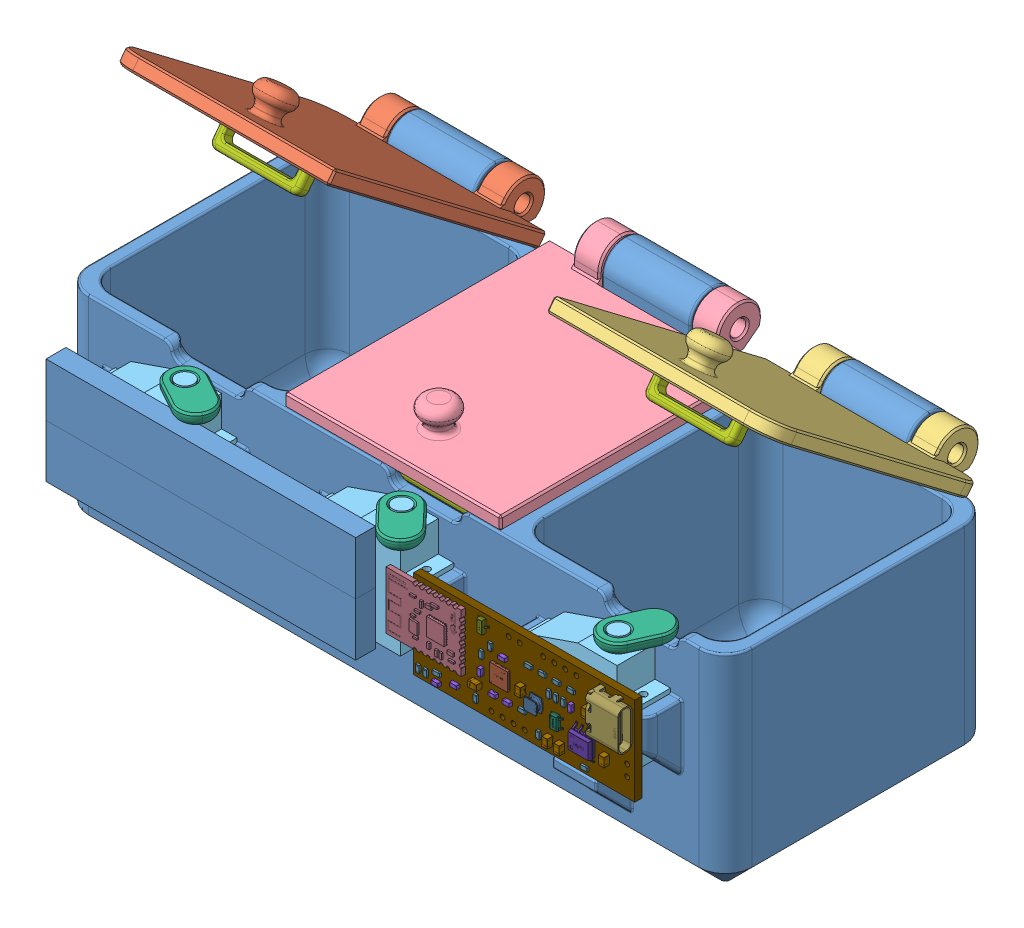
SolidWorks assembly 装配, configuration 默认. Lengths in mm.
Overall size (150 94.48 83.55).
139 component instances, 22 part files, 42 mates.
Components (placement in the parent):
- 盒子-1: 盒子 [默认] at (-79.9939 -35.3926 182.681) size (150 58 75.91)
- 边盖-1: 边盖 [默认] at (-29.4939 51.285 172.8919) x (0 -0.604443 -0.796648) z (1 0 0) size (67.2 9.8 50.35)
- 镜向边盖-2: 镜向边盖 [默认] at (19.5061 51.285 172.8919) x (0 -0.604443 -0.796648) z (1 0 0) size (67.2 9.8 50.35)
- 中盖-1: 中盖 [默认] at (19.3061 12.7974 182.671) x (0 0 -1) z (1 0 0) size (67.2 9.8 48.9)
- 小舵机-1: 小舵机 [默认] at (-64.3939 -14.1926 191.281) size (27.5 25.65 8.6)
- 小舵机-2: 小舵机 [默认] at (33.6061 -14.1926 191.281) size (27.5 25.65 8.6)
- 小舵机-3: 小舵机 [默认] at (-15.3939 -14.1926 191.281) size (27.5 25.65 8.6)
- 锁-1: 锁 [默认] at (-47.8939 8.4574 186.981) x (0 1 0) z (0.479802 0 -0.877377) size (3 14 8)
- 锁-2: 锁 [默认] at (50.1061 8.4574 186.981) x (0 1 0) z (-0.912479 0 -0.409122) size (3 14 8)
- 锁-3: 锁 [默认] at (1.1061 8.4574 186.981) x (0 1 0) z (0.725826 0 -0.687879) size (3 14 8)
- 电路盒-1: 电路盒 [默认] at (64.0061 -30.3926 200.181) x (-1 0 0) z (0 0 -1) size (138 47.35 22.96) (hidden)
- 盖子锁口-1: 盖子锁口 [默认] at (-56.9939 43.6916 170.4941) x (1 0 0) z (0 -0.796648 0.604443) size (20 3 6.1)
- 盖子锁口-2: 盖子锁口 [默认] at (41.0061 43.6916 170.4941) x (1 0 0) z (0 -0.796648 0.604443) size (20 3 6.1)
- 盖子锁口-3: 盖子锁口 [默认] at (-7.9939 8.1974 176.171) x (1 0 0) z (0 -1 0) size (20 3 6.1)
- 3D_BOX_2024-11-24-1: 3D_BOX_2024-11-24 [默认] at (10.7267 5.7947 191.781) size (55.21 19.97 4.86)
  - 3D_BOX_2024-11-24.step-1: 3D_BOX_2024-11-24.step [默认] at origin size (56.98 23.31 10.6)
    - 3yDE-C2.step-1: 3yDE-C2.step [默认] at (21.082 -14.478 1.6001) x (-1 0 0) z (0 0 1) size (1.6 0.8 0.8)
      - C0603.step-1: C0603.step [默认] at origin size (1.6 0.8 0.8)
        - SOLID.step-1: SOLID.step [默认] at origin size (1.6 0.8 0.8)
    - 3yDE-C3.step-1: 3yDE-C3.step [默认] at (14.986 -11.43 1.6001) x (0 -1 0) z (0 0 1) size (1.6 0.8 0.8)
      - C0603.step-1: C0603.step [默认] at origin size (1.6 0.8 0.8)
        - SOLID.step-1: SOLID.step [默认] at origin size (1.6 0.8 0.8)
    - 3yDE-C4.step-1: 3yDE-C4.step [默认] at (20.066 -6.223 1.6001) x (-1 0 0) z (0 0 1) size (1.6 0.8 0.8)
      - C0603.step-1: C0603.step [默认] at origin size (1.6 0.8 0.8)
        - SOLID.step-1: SOLID.step [默认] at origin size (1.6 0.8 0.8)
    - 3yDE-C5.step-1: 3yDE-C5.step [默认] at (9.144 -17.018 1.6001) x (-1 0 0) z (0 0 1) size (1.6 0.8 0.8)
      - C0603.step-1: C0603.step [默认] at origin size (1.6 0.8 0.8)
        - SOLID.step-1: SOLID.step [默认] at origin size (1.6 0.8 0.8)
    - 3yDE-C6.step-1: 3yDE-C6.step [默认] at (4.953 -18.669 1.6001) x (-1 0 0) z (0 0 1) size (1.6 0.8 0.8)
      - C0603.step-1: C0603.step [默认] at origin size (1.6 0.8 0.8)
        - SOLID.step-1: SOLID.step [默认] at origin size (1.6 0.8 0.8)
    - 3yDE-C11.step-1: 3yDE-C11.step [默认] at (35.4331 -8.255 1.6001) x (0 -1 0) z (0 0 1) size (1.6 0.8 0.8)
      - C0603.step-1: C0603.step [默认] at origin size (1.6 0.8 0.8)
        - SOLID.step-1: SOLID.step [默认] at origin size (1.6 0.8 0.8)
    - 3yDE-C1.step-1: 3yDE-C1.step [默认] at (17.907 -14.478 1.6001) size (1.6 0.8 0.8)
      - C0603.step-1: C0603.step [默认] at origin size (1.6 0.8 0.8)
        - SOLID.step-1: SOLID.step [默认] at origin size (1.6 0.8 0.8)
    - 3yDE-C8.step-1: 3yDE-C8.step [默认] at (24.257 -10.287 1.6001) x (0 -1 0) z (0 0 1) size (2 1.3 1.3)
      - C0805.step-1: C0805.step [默认] at origin size (2 1.3 1.3)
        - SOLID-0.step-1: SOLID-0.step [默认] at origin size (2 1.3 1.3)
    - 3yDE-C9.step-1: 3yDE-C9.step [默认] at (33.0201 -17.272 1.6001) x (0 1 0) z (0 0 1) size (2 1.3 1.3)
      - C0805.step-1: C0805.step [默认] at origin size (2 1.3 1.3)
        - SOLID-0.step-1: SOLID-0.step [默认] at origin size (2 1.3 1.3)
    - 3yDE-C10.step-1: 3yDE-C10.step [默认] at (30.3531 -17.272 1.6001) x (0 1 0) z (0 0 1) size (2 1.3 1.3)
      - C0805.step-1: C0805.step [默认] at origin size (2 1.3 1.3)
        - SOLID-0.step-1: SOLID-0.step [默认] at origin size (2 1.3 1.3)
    - 3yDE-C12.step-1: 3yDE-C12.step [默认] at (39.2431 -7.112 1.6001) x (0 -1 0) z (0 0 1) size (2 1.3 1.3)
      - C0805.step-1: C0805.step [默认] at origin size (2 1.3 1.3)
        - SOLID-0.step-1: SOLID-0.step [默认] at origin size (2 1.3 1.3)
    - 3yDE-C13.step-1: 3yDE-C13.step [默认] at (43.1801 -14.478 1.6001) x (0 1 0) z (0 0 1) size (2 1.3 1.3)
      - C0805.step-1: C0805.step [默认] at origin size (2 1.3 1.3)
        - SOLID-0.step-1: SOLID-0.step [默认] at origin size (2 1.3 1.3)
    - 3yDE-C7.step-1: 3yDE-C7.step [默认] at (13.97 -14.351 1.6001) x (-1 0 0) z (0 0 1) size (2 1.3 1.3)
      - C0805.step-1: C0805.step [默认] at origin size (2 1.3 1.3)
        - SOLID-0.step-1: SOLID-0.step [默认] at origin size (2 1.3 1.3)
    - 3yDE-S1.step-1: 3yDE-S1.step [默认] at (32.5121 -1.778 1.6001) size (12.5 5.7 10)
      - CONN-TH_4P-P2.50_4PIN.step-1: CONN-TH_4P-P2.50_4PIN.step [默认] at origin size (12.5 5.7 10)
        - COMPOUND.step-1: COMPOUND.step [默认] at origin size (12.5 5.7 10) (hidden)
    - 3yDE-DOWNLOAD1.step-1: 3yDE-DOWNLOAD1.step [默认] at (20.828 -18.288 1.6001) x (-1 0 0) z (0 0 1) size (12.5 5.7 10)
      - CONN-TH_4P-P2.50_4PIN.step-1: CONN-TH_4P-P2.50_4PIN.step [默认] at origin size (12.5 5.7 10)
        - COMPOUND.step-1: COMPOUND.step [默认] at origin size (12.5 5.7 10) (hidden)
    - 3yDE-L1.step-1: 3yDE-L1.step [默认] at (27.3051 -11.557 1.6001) x (0 -1 0) z (0 0 1) size (3 3 1.52)
      - IND-SMD_L3.0-W3.0_FNR30XXS.step-1: IND-SMD_L3.0-W3.0_FNR30XXS.step [默认] at origin size (3 3 1.52)
        - SOLID-1.step-1: SOLID-1.step [默认] at origin size (3 3 1.52)
    - 3yDE-U2.step-1: 3yDE-U2.step [默认] at (19.304 -10.287 1.6001) size (4.03 4.03 0.61)
      - UFQFPN-28_L4.0-W4.0-P0.50-BL.step-1: UFQFPN-28_L4.0-W4.0-P0.50-BL.step [默认] at origin size (4.03 4.03 0.61)
        - SOLID-2.step-1: SOLID-2.step [默认] at origin size (4.03 4.03 0.61)
    - 3yDE-BAT1.step-1: 3yDE-BAT1.step [默认] at (47.7521 -14.605 1.6001) x (0 1 0) z (0 0 1) size (7.5 5.9 10.6)
      - CONN-TH_2P-P2.50_HX25003-2A.step-1: CONN-TH_2P-P2.50_HX25003-2A.step [默认] at origin size (7.5 5.9 10.6)
        - COMPOUND-3.step-1: COMPOUND-3.step [默认] at origin size (7.5 5.9 10.6) (hidden)
    - 3yDE-SPOWER1.step-1: 3yDE-SPOWER1.step [默认] at (22.225 -1.778 1.6001) x (-1 0 0) z (0 0 1) size (7.5 5.9 10.6)
      - CONN-TH_2P-P2.50_HX25003-2A.step-1: CONN-TH_2P-P2.50_HX25003-2A.step [默认] at origin size (7.5 5.9 10.6)
        - COMPOUND-3.step-1: COMPOUND-3.step [默认] at origin size (7.5 5.9 10.6) (hidden)
    - 3yDE-USB1.step-1: 3yDE-USB1.step [默认] at (43.9421 -5.334 1.6001) x (0 1 0) z (0 0 1) size (8.95 7.58 4.16)
      - USB-C-SMD_TYPE-C-6PIN-2MD-073.step-1: USB-C-SMD_TYPE-C-6PIN-2MD-073.step [默认] at origin size (8.95 7.58 4.16)
        - COMPOUND-4.step-1: COMPOUND-4.step [默认] at origin size (8.95 7.58 4.16)
    - 3yDE-U1.step-1: 3yDE-U1.step [默认] at (5.969 -7.493 1.6001) x (0 1 0) z (0 0 1) size (13 17 1.62)
      - BULETM-SMD_ZX-D30.step-1: BULETM-SMD_ZX-D30.step [默认] at origin size (13 17 1.62)
        - SOLID-5.step-1: SOLID-5.step [默认] at origin size (13 17 1.62)
    - 3yDE-R2.step-1: 3yDE-R2.step [默认] at (24.2672 -14.4989 1.6001) x (-1 0 0) z (0 0 1) size (1.62 0.81 0.45)
      - R0603.step-1: R0603.step [默认] at origin size (1.62 0.81 0.45)
        - COMPOUND-6.step-1: COMPOUND-6.step [默认] at origin size (1.62 0.81 0.45)
    - 3yDE-R3.step-1: 3yDE-R3.step [默认] at (4.953 -16.891 1.6001) x (-1 0 0) z (0 0 1) size (1.62 0.81 0.45)
      - R0603.step-1: R0603.step [默认] at origin size (1.62 0.81 0.45)
        - COMPOUND-6.step-1: COMPOUND-6.step [默认] at origin size (1.62 0.81 0.45)
    - 3yDE-R4.step-1: 3yDE-R4.step [默认] at (0.762 -18.034 1.6001) x (0 1 0) z (0 0 1) size (1.62 0.81 0.45)
      - R0603.step-1: R0603.step [默认] at origin size (1.62 0.81 0.45)
        - COMPOUND-6.step-1: COMPOUND-6.step [默认] at origin size (1.62 0.81 0.45)
    - 3yDE-R5.step-1: 3yDE-R5.step [默认] at (2.413 -18.034 1.6001) x (0 1 0) z (0 0 1) size (1.62 0.81 0.45)
      - R0603.step-1: R0603.step [默认] at origin size (1.62 0.81 0.45)
        - COMPOUND-6.step-1: COMPOUND-6.step [默认] at origin size (1.62 0.81 0.45)
    - 3yDE-R6.step-1: 3yDE-R6.step [默认] at (13.716 -17.399 1.6001) x (0 1 0) z (0 0 1) size (1.62 0.81 0.45)
      - R0603.step-1: R0603.step [默认] at origin size (1.62 0.81 0.45)
        - COMPOUND-6.step-1: COMPOUND-6.step [默认] at origin size (1.62 0.81 0.45)
    - 3yDE-R7.step-1: 3yDE-R7.step [默认] at (27.9401 -17.399 1.6001) x (0 1 0) z (0 0 1) size (1.62 0.81 0.45)
      - R0603.step-1: R0603.step [默认] at origin size (1.62 0.81 0.45)
        - COMPOUND-6.step-1: COMPOUND-6.step [默认] at origin size (1.62 0.81 0.45)
    - 3yDE-R8.step-1: 3yDE-R8.step [默认] at (35.3061 -5.08 1.6001) x (-1 0 0) z (0 0 1) size (1.62 0.81 0.45)
      - R0603.step-1: R0603.step [默认] at origin size (1.62 0.81 0.45)
        - COMPOUND-6.step-1: COMPOUND-6.step [默认] at origin size (1.62 0.81 0.45)
    - 3yDE-R9.step-1: 3yDE-R9.step [默认] at (32.0041 -5.08 1.6001) x (-1 0 0) z (0 0 1) size (1.62 0.81 0.45)
      - R0603.step-1: R0603.step [默认] at origin size (1.62 0.81 0.45)
        - COMPOUND-6.step-1: COMPOUND-6.step [默认] at origin size (1.62 0.81 0.45)
    - 3yDE-R10.step-1: 3yDE-R10.step [默认] at (28.8291 -5.08 1.6001) x (-1 0 0) z (0 0 1) size (1.62 0.81 0.45)
      - R0603.step-1: R0603.step [默认] at origin size (1.62 0.81 0.45)
        - COMPOUND-6.step-1: COMPOUND-6.step [默认] at origin size (1.62 0.81 0.45)
    - 3yDE-R11.step-1: 3yDE-R11.step [默认] at (25.6541 -5.08 1.6001) x (-1 0 0) z (0 0 1) size (1.62 0.81 0.45)
      - R0603.step-1: R0603.step [默认] at origin size (1.62 0.81 0.45)
        - COMPOUND-6.step-1: COMPOUND-6.step [默认] at origin size (1.62 0.81 0.45)
    - 3yDE-R12.step-1: 3yDE-R12.step [默认] at (30.2261 -8.255 1.6001) x (0 -1 0) z (0 0 1) size (1.62 0.81 0.45)
      - R0603.step-1: R0603.step [默认] at origin size (1.62 0.81 0.45)
        - COMPOUND-6.step-1: COMPOUND-6.step [默认] at origin size (1.62 0.81 0.45)
    - 3yDE-R13.step-1: 3yDE-R13.step [默认] at (31.8771 -8.255 1.6001) x (0 1 0) z (0 0 1) size (1.62 0.81 0.45)
      - R0603.step-1: R0603.step [默认] at origin size (1.62 0.81 0.45)
        - COMPOUND-6.step-1: COMPOUND-6.step [默认] at origin size (1.62 0.81 0.45)
    - 3yDE-R16.step-1: 3yDE-R16.step [默认] at (38.3541 -18.669 1.6001) x (-1 0 0) z (0 0 1) size (1.62 0.81 0.45)
      - R0603.step-1: R0603.step [默认] at origin size (1.62 0.81 0.45)
        - COMPOUND-6.step-1: COMPOUND-6.step [默认] at origin size (1.62 0.81 0.45)
    - 3yDE-R17.step-1: 3yDE-R17.step [默认] at (17.018 -5.588 1.6001) x (0 1 0) z (0 0 1) size (1.62 0.81 0.45)
      - R0603.step-1: R0603.step [默认] at origin size (1.62 0.81 0.45)
        - COMPOUND-6.step-1: COMPOUND-6.step [默认] at origin size (1.62 0.81 0.45)
    - 3yDE-R14.step-1: 3yDE-R14.step [默认] at (33.5281 -8.255 1.6001) x (0 -1 0) z (0 0 1) size (1.62 0.81 0.45)
      - R0603.step-1: R0603.step [默认] at origin size (1.62 0.81 0.45)
        - COMPOUND-6.step-1: COMPOUND-6.step [默认] at origin size (1.62 0.81 0.45)
    - 3yDE-R1.step-1: 3yDE-R1.step [默认] at (14.986 -8.128 1.6001) x (0 -1 0) z (0 0 1) size (1.62 0.81 0.45)
      - R0603.step-1: R0603.step [默认] at origin size (1.62 0.81 0.45)
        - COMPOUND-6.step-1: COMPOUND-6.step [默认] at origin size (1.62 0.81 0.45)
    - 3yDE-U3.step-1: 3yDE-U3.step [默认] at (32.0041 -12.7 1.6001) x (0 -1 0) z (0 0 1) size (2.9 2.81 1.05)
      - TSOT-25_L2.9-W1.6-P0.95-BL.step-1: TSOT-25_L2.9-W1.6-P0.95-BL.step [默认] at origin size (2.9 2.81 1.05)
        - COMPOUND-7.step-1: COMPOUND-7.step [默认] at origin size (2.9 2.81 1.05)
    - 3yDE-Q1.step-1: 3yDE-Q1.step [默认] at (15.367 -2.159 1.6001) x (-1 0 0) z (0 0 1) size (2.5 2.89 1.05)
      - SOT-23-3_L2.9-W1.3-P1.90-LS2.4-BR.step-1: SOT-23-3_L2.9-W1.3-P1.90-LS2.4-BR.step [默认] at origin size (2.5 2.89 1.05)
        - COMPOUND-8.step-1: COMPOUND-8.step [默认] at origin size (2.5 2.89 1.05)
    - 3yDE-U4.step-1: 3yDE-U4.step [默认] at (38.3541 -13.716 1.6001) size (4.9 6.1 1.7)
      - ESOP-8_L4.9-W3.9-P1.27-LS6.0-BL-EP.step-1: ESOP-8_L4.9-W3.9-P1.27-LS6.0-BL-EP.step [默认] at origin size (4.9 6.1 1.7)
        - COMPOUND-9.step-1: COMPOUND-9.step [默认] at origin size (4.9 6.1 1.7)
    - Board.step-1: Board.step [默认] at origin size (49.97 19.97 1.6)
- 电池-1: 电池 [默认] at (-70.4939 8.4574 195.781) x (1 0 0) z (0 1 0) size (70 4.5 12)
- 电池-2: 电池 [默认] at (-70.4939 -3.5426 195.781) x (1 0 0) z (0 1 0) size (70 4.5 12)
Mates (geometry in assembly coordinates):
- 重合2: coincident aligned: plane of 盒子-1 through (-79.9939 -32.3926 182.681) normal (-1 0 0); plane of 边盖-1 through (-79.9939 53.675 171.0785) normal (-1 0 0)
- 同心1: concentric anti-aligned: cylinder of 盒子-1 through (70.0061 17.5074 120.581) axis (-1 0 0) radius 1.5; cylinder of 边盖-1 through (-79.9939 17.5074 120.581) axis (1 0 0) radius 1.8
- 同心2: concentric anti-aligned: cylinder of 盒子-1 through (70.0061 17.5074 120.581) axis (-1 0 0) radius 1.5; cylinder of 中盖-1 through (-31.1939 17.5074 120.581) axis (1 0 0) radius 1.8
- 距离1: distance = 0.1 mm anti-aligned: plane of 中盖-1 through (5.1061 5.7974 122.671) normal (-1 0 0); plane of 盒子-1 through (5.0061 22.6074 122.681) normal (1 0 0)
- LimitAngle1: limit planar angle = 0.649066 rad anti-aligned: plane of 边盖-1 through (-29.4939 51.285 172.8919) normal (0 -0.796648 0.604443); plane of 盒子-1 through (-79.9939 12.6074 182.681) normal (0 1 0)
- LimitAngle2: limit planar angle = 0 rad anti-aligned: plane of 中盖-1 through (19.3061 12.7974 182.671) normal (0 -1 0); plane of 盒子-1 through (-79.9939 12.6074 182.681) normal (0 1 0)
- 重合6: coincident anti-aligned: plane of 盒子-1 through (-79.9939 -32.3926 182.681) normal (0 0 1); plane of 小舵机-1 through (-64.3939 1.0074 182.681) normal (0 0 -1)
- 重合7: coincident anti-aligned: plane of 盒子-1 through (-64.4939 0.5074 191.281) normal (0 1 0); plane of 小舵机-1 through (-64.3939 0.5074 182.681) normal (0 -1 0)
- 距离2: distance = 0.1 mm anti-aligned: plane of 小舵机-1 through (-43.8939 1.0074 191.281) normal (1 0 0); plane of 盒子-1 through (-43.7939 0.5074 191.281) normal (-1 0 0)
- 重合9: coincident anti-aligned: plane of 盒子-1 through (5.2061 0.5074 191.281) normal (0 1 0); plane of 小舵机-3 through (5.1061 0.5074 182.681) normal (0 -1 0)
- 同心3: concentric aligned: circle of 盒子-1; cylinder of 小舵机-3 through (6.7261 -7.0926 186.981) axis (0 1 0) radius 0.8
- 同心4: concentric aligned: cylinder of 盒子-1 through (-17.0139 -7.4926 186.981) axis (0 1 0) radius 0.7; cylinder of 小舵机-3 through (-17.0139 -7.0926 186.981) axis (0 1 0) radius 0.8
- 重合10: coincident anti-aligned: plane of 盒子-1 through (33.5061 0.5074 191.281) normal (0 1 0); plane of 小舵机-2 through (54.1061 0.5074 182.681) normal (0 -1 0)
- 同心5: concentric aligned: circle of 盒子-1; circle of 小舵机-2
- 同心6: concentric aligned: cylinder of 盒子-1 through (31.9861 -7.4926 186.981) axis (0 1 0) radius 0.7; cylinder of 小舵机-2 through (31.9861 -7.0926 186.981) axis (0 1 0) radius 0.8
- 同心7: concentric aligned: cylinder of 小舵机-1 through (-47.8939 11.4574 186.981) axis (0 -1 0) radius 2; cylinder of 锁-1 through (-47.8939 11.4574 186.981) axis (0 -1 0) radius 2
- 重合12: coincident anti-aligned: plane of 小舵机-3 through (5.1061 8.4574 182.681) normal (0 1 0); plane of 锁-3 through (1.1061 8.4574 186.981) normal (0 -1 0)
- 重合13: coincident anti-aligned: plane of 小舵机-2 through (54.1061 8.4574 182.681) normal (0 1 0); plane of 锁-2 through (50.1061 8.4574 186.981) normal (0 -1 0)
- 同心8: concentric aligned: cylinder of 小舵机-2 through (50.1061 11.4574 186.981) axis (0 -1 0) radius 2; cylinder of 锁-2 through (50.1061 11.4574 186.981) axis (0 -1 0) radius 2
- 同心9: concentric aligned: cylinder of 小舵机-3 through (1.1061 11.4574 186.981) axis (0 -1 0) radius 2; cylinder of 锁-3 through (1.1061 11.4574 186.981) axis (0 -1 0) radius 2
- 重合14: coincident anti-aligned: plane of 盒子-1 through (-79.9939 -32.3926 182.681) normal (0 0 1); plane of 电路盒-1 through (64.0061 -30.3926 182.681) normal (0 0 -1)
- 重合15: coincident: line of 盒子-1 through (-73.9939 -30.3926 182.681) axis (1 0 0); plane of 电路盒-1 through (64.0061 -30.3926 197.181) normal (0 -1 0)
- 重合16: coincident anti-aligned: line of 盒子-1 through (64.0061 -30.3926 182.681) axis (0 1 0); line of 电路盒-1 through (64.0061 9.0174 182.681) axis (0 -1 0)
- 重合17: coincident aligned: plane of 锁-1 through (-47.8939 11.4574 186.981) normal (0 1 0); plane of 锁-3 through (1.1061 11.4574 186.981) normal (0 1 0)
- 重合18: coincident anti-aligned: plane of 边盖-1 through (-29.4939 52.48 171.9852) normal (0 -0.796648 0.604443); plane of 盖子锁口-1 through (-56.9939 50.3645 169.1969) normal (0 0.796648 -0.604443)
- 距离4: distance = 0.1 mm anti-aligned: plane of 盖子锁口-1 through (-36.9939 45.5049 172.884) normal (1 0 0); plane of 边盖-1 through (-36.8939 50.4249 169.2766) normal (-1 0 0)
- 距离5: distance = 0.1 mm anti-aligned: plane of 盖子锁口-1 through (-56.9939 45.5049 172.884) normal (0 0.604443 0.796648); plane of 边盖-1 through (-57.0939 50.4249 169.2766) normal (0 -0.604443 -0.796648)
- 距离6: distance = 0.1 mm anti-aligned: plane of 盖子锁口-2 through (41.0061 45.5049 172.884) normal (0 0.604443 0.796648); plane of 镜向边盖-2 through (61.1061 50.4249 169.2766) normal (0 -0.604443 -0.796648)
- 距离7: distance = 0.1 mm anti-aligned: plane of 盖子锁口-2 through (61.0061 45.5049 172.884) normal (1 0 0); plane of 镜向边盖-2 through (61.1061 50.4249 169.2766) normal (-1 0 0)
- 重合24: coincident anti-aligned: plane of 镜向边盖-2 through (19.5061 52.48 171.9852) normal (0 -0.796648 0.604443); plane of 盖子锁口-2 through (41.0061 50.3645 169.1969) normal (0 0.796648 -0.604443)
- 重合25: coincident anti-aligned: plane of 中盖-1 through (19.3061 14.2974 182.671) normal (0 -1 0); plane of 盖子锁口-3 through (-7.9939 14.2974 179.171) normal (0 1 0)
- 距离8: distance = 0.1 mm anti-aligned: plane of 盖子锁口-3 through (-7.9939 8.1974 179.171) normal (0 0 1); plane of 中盖-1 through (-8.0939 14.2974 179.271) normal (0 0 -1)
- 距离9: distance = 0.1 mm anti-aligned: plane of 盖子锁口-3 through (12.0061 8.1974 179.171) normal (1 0 0); plane of 中盖-1 through (12.1061 14.2974 179.271) normal (-1 0 0)
- 距离10: distance = 0.5 mm anti-aligned: plane of 小舵机-3 through (-15.3939 1.0074 191.281) normal (0 0 1); plane of 3D_BOX_2024-11-24-1/3D_BOX_2024-11-24.step-1/Board.step-1 through (35.2187 -4.2053 191.781) normal (0 0 -1)
- 重合27: coincident aligned: plane of 盒子-1 through (60.2061 0.5074 191.281) normal (1 0 0); plane of 3D_BOX_2024-11-24-1/3D_BOX_2024-11-24.step-1/Board.step-1 through (60.2061 5.782 191.781) normal (1 0 0)
- 重合28: coincident aligned: plane of 小舵机-2 through (33.6061 -14.1926 191.281) normal (0 -1 0); plane of 3D_BOX_2024-11-24-1/3D_BOX_2024-11-24.step-1/Board.step-1 through (60.2061 -14.1926 191.781) normal (0 -1 0)
- 重合29: coincident anti-aligned: plane of 小舵机-1 through (-64.3939 1.0074 191.281) normal (0 0 1); plane of 电池-1 through (-70.4939 8.4574 191.281) normal (0 0 -1)
- 重合30: coincident anti-aligned: plane of 小舵机-1 through (-64.3939 1.0074 191.281) normal (0 0 1); plane of 电池-2 through (-70.4939 -3.5426 191.281) normal (0 0 -1)
- 重合32: coincident aligned: plane of 盒子-1 through (-70.4939 0.5074 191.281) normal (-1 0 0); plane of 电池-1 through (-70.4939 8.4574 191.281) normal (-1 0 0)
- 重合33: coincident aligned: plane of 盒子-1 through (-70.4939 0.5074 191.281) normal (-1 0 0); plane of 电池-2 through (-70.4939 -3.5426 191.281) normal (-1 0 0)
- 重合34: coincident aligned: plane of 小舵机-1 through (-43.8939 8.4574 182.681) normal (0 1 0); plane of 电池-1 through (-70.4939 8.4574 191.281) normal (0 1 0)
- 重合35: coincident anti-aligned: plane of 电池-1 through (-70.4939 -3.5426 191.281) normal (0 -1 0); plane of 电池-2 through (-70.4939 -3.5426 191.281) normal (0 1 0)
